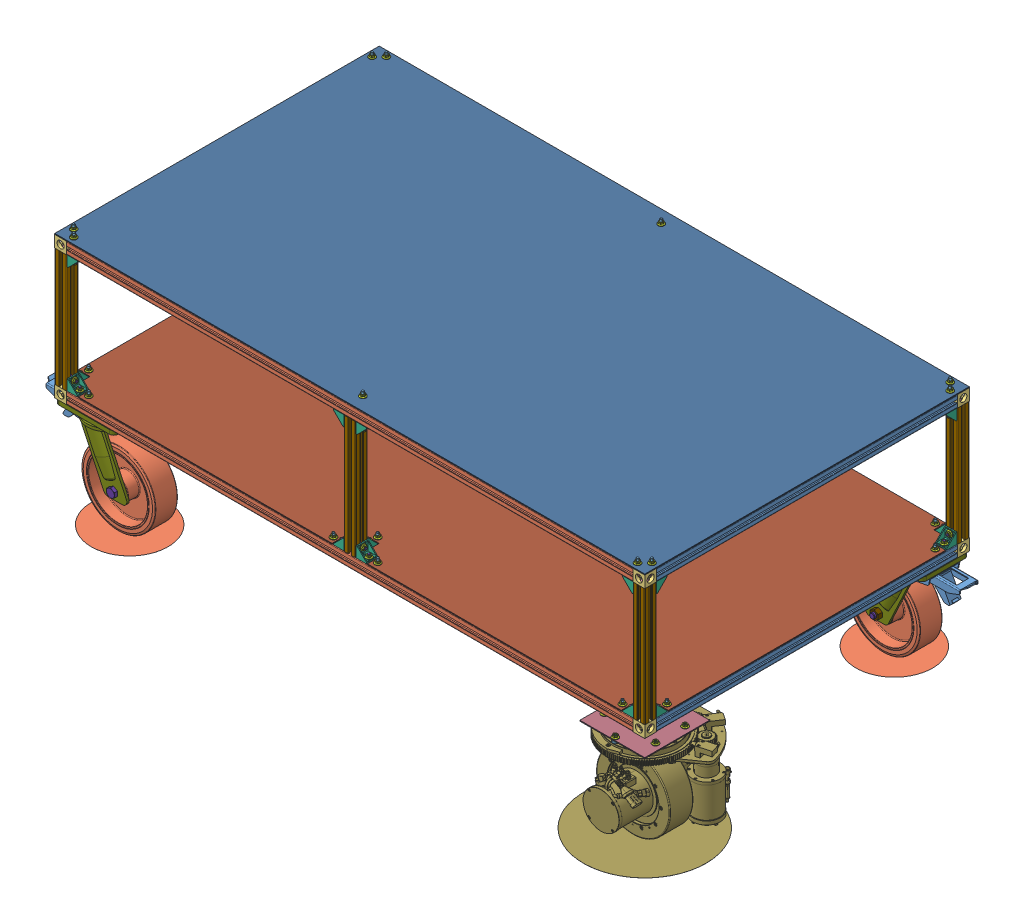
SolidWorks assembly totale, configuration Default. Lengths in mm.
Overall size (2298.39 831.64 1387.9).
545 component instances, 20 part files, 36 mates.
Components (placement in the parent):
- body-1: body [Default] at (-233.7628 101.484 2240) size (2000 498.7 1100)
  - body_skeleton-1: body_skeleton [Default] at (-1.581 -195.357 0) size (2000 480 1100)
    - Piano_base-1: Piano_base [Default] at (1030.9122 10.7283 790) size (2000 66.8 1100)
      - profilato_1020-1: profilato_1020 [Default] at (-20 -20 -1540) size (40 40 1020)
      - profilato_1920-1: profilato_1920 [Default] at (-40 -20 -1560) x (0 1 0) z (-1 0 0) size (40 40 1920)
      - profilato_1020-2: profilato_1020 [Default] at (-1980 -20 -520) x (0 -1 0) z (0 0 -1) size (40 40 1020)
      - profilato_1920-2: profilato_1920 [Default] at (-40 -20 -500) x (0 0 -1) z (-1 0 0) size (40 40 1920)
      - cubic_joint_screws-1: cubic_joint_screws [Default] at (-11.6556 -20 -1565.4929) x (0 0 1) z (0 -1 0) size (66.8 66.8 66.8)
        - cubic_joint_3-1: cubic_joint_3 [Default] at (25.4929 8.3444 0) size (40 40 40)
        - CORE_SCREW_S12X30_T50-1: CORE_SCREW_S12X30_T50 [Default] at (27.9929 8.3444 0) x (0 -0.924225 -0.381849) z (1 0 0) size (19.6 19.6 35.7)
        - CORE_SCREW_S12X30_T50-2: CORE_SCREW_S12X30_T50 [Default] at (5.4929 30.8444 0) x (-0.999796 0 0.020189) z (0 1 0) size (19.6 19.6 35.7)
        - CORE_SCREW_S12X30_T50-3: CORE_SCREW_S12X30_T50 [Default] at (5.4929 8.3444 -22.5) x (-0.923728 -0.383049 0) z (0 0 -1) size (19.6 19.6 35.7)
      - cubic_joint_screws-2: cubic_joint_screws [Default] at (-1985.4929 -20 -1568.3444) x (1 0 0) z (0 -1 0) size (66.8 66.8 66.8)
        - cubic_joint_3-1: cubic_joint_3 [Default] at (25.4929 8.3444 0) size (40 40 40)
        - CORE_SCREW_S12X30_T50-1: CORE_SCREW_S12X30_T50 [Default] at (27.9929 8.3444 0) x (0 -0.924225 -0.381849) z (1 0 0) size (19.6 19.6 35.7)
        - CORE_SCREW_S12X30_T50-2: CORE_SCREW_S12X30_T50 [Default] at (5.4929 30.8444 0) x (-0.999796 0 0.020189) z (0 1 0) size (19.6 19.6 35.7)
        - CORE_SCREW_S12X30_T50-3: CORE_SCREW_S12X30_T50 [Default] at (5.4929 8.3444 -22.5) x (-0.923728 -0.383049 0) z (0 0 -1) size (19.6 19.6 35.7)
      - cubic_joint_screws-3: cubic_joint_screws [Default] at (-11.6556 -25.4929 -500) x (0 1 0) z (0 0 1) size (66.8 66.8 66.8)
        - cubic_joint_3-1: cubic_joint_3 [Default] at (25.4929 8.3444 0) size (40 40 40)
        - CORE_SCREW_S12X30_T50-1: CORE_SCREW_S12X30_T50 [Default] at (27.9929 8.3444 0) x (0 -0.924225 -0.381849) z (1 0 0) size (19.6 19.6 35.7)
        - CORE_SCREW_S12X30_T50-2: CORE_SCREW_S12X30_T50 [Default] at (5.4929 30.8444 0) x (-0.999796 0 0.020189) z (0 1 0) size (19.6 19.6 35.7)
        - CORE_SCREW_S12X30_T50-3: CORE_SCREW_S12X30_T50 [Default] at (5.4929 8.3444 -22.5) x (-0.923728 -0.383049 0) z (0 0 -1) size (19.6 19.6 35.7)
      - cubic_joint_screws-4: cubic_joint_screws [Default] at (-1985.4929 -28.3444 -500) size (66.8 66.8 66.8)
        - cubic_joint_3-1: cubic_joint_3 [Default] at (25.4929 8.3444 0) size (40 40 40)
        - CORE_SCREW_S12X30_T50-1: CORE_SCREW_S12X30_T50 [Default] at (27.9929 8.3444 0) x (0 -0.924225 -0.381849) z (1 0 0) size (19.6 19.6 35.7)
        - CORE_SCREW_S12X30_T50-2: CORE_SCREW_S12X30_T50 [Default] at (5.4929 30.8444 0) x (-0.999796 0 0.020189) z (0 1 0) size (19.6 19.6 35.7)
        - CORE_SCREW_S12X30_T50-3: CORE_SCREW_S12X30_T50 [Default] at (5.4929 8.3444 -22.5) x (-0.923728 -0.383049 0) z (0 0 -1) size (19.6 19.6 35.7)
      - longherone_h-4: longherone_h [Default] at (-1507.1648 -11.1801 -790) size (112 40 1043.4)
        - profilato_1020-1: profilato_1020 [Default] at (33.8348 -8.8199 -750) size (40 40 1020)
        - T_BOLT-1: T_BOLT [Default] at (33.8348 -8.8199 276) x (0 -1 0) z (0 0 1) size (19.4 8.5 30.4)
        - T_BOLT-2: T_BOLT [Default] at (33.8348 -8.8199 -756) x (0 -1 0) z (0 0 -1) size (19.4 8.5 30.4)
        - Bracket_40_40_set-2: Bracket_40_40_set [Default] at (-7.7665 -12.3804 -732) x (0 1 0) z (0 0 1) size (38 47.7 51.56)
          - bracket_40_40-1: bracket_40_40 [Default] at (-15.4395 -1.6013 2) size (38 36 36)
          - FLANGE_NUT_M8-3: FLANGE_NUT_M8 [Default] at (3.5605 3.5487 -12.5) size (21 21 8)
          - T_BOLT_short-4: T_BOLT_short [Default] at (3.5605 3.5487 -24) x (-1 0 0) z (0 0 -1) size (19.4 8.5 26.9)
          - FLANGE_NUT_M8-4: FLANGE_NUT_M8 [Default] at (3.5605 -16.1013 7.15) x (0.797177 0 0.603746) z (0 1 0) size (21 21 8)
          - T_BOLT_short-5: T_BOLT_short [Default] at (3.5605 -27.6013 7.15) x (-1 0 0) z (0 -1 0) size (19.4 8.5 26.9)
        - Bracket_40_40_set-3: Bracket_40_40_set [Default] at (75.436 -5.2593 -732) x (0 -1 0) z (0 0 1) size (38 47.7 51.56)
          - bracket_40_40-1: bracket_40_40 [Default] at (-15.4395 -1.6013 2) size (38 36 36)
          - FLANGE_NUT_M8-3: FLANGE_NUT_M8 [Default] at (3.5605 3.5487 -12.5) size (21 21 8)
          - T_BOLT_short-4: T_BOLT_short [Default] at (3.5605 3.5487 -24) x (-1 0 0) z (0 0 -1) size (19.4 8.5 26.9)
          - FLANGE_NUT_M8-4: FLANGE_NUT_M8 [Default] at (3.5605 -16.1013 7.15) x (0.797177 0 0.603746) z (0 1 0) size (21 21 8)
          - T_BOLT_short-5: T_BOLT_short [Default] at (3.5605 -27.6013 7.15) x (-1 0 0) z (0 -1 0) size (19.4 8.5 26.9)
        - Bracket_40_40_set-4: Bracket_40_40_set [Default] at (75.436 -12.3804 252) x (0 1 0) z (0 0 -1) size (38 47.7 51.56)
          - bracket_40_40-1: bracket_40_40 [Default] at (-15.4395 -1.6013 2) size (38 36 36)
          - FLANGE_NUT_M8-3: FLANGE_NUT_M8 [Default] at (3.5605 3.5487 -12.5) size (21 21 8)
          - T_BOLT_short-4: T_BOLT_short [Default] at (3.5605 3.5487 -24) x (-1 0 0) z (0 0 -1) size (19.4 8.5 26.9)
          - FLANGE_NUT_M8-4: FLANGE_NUT_M8 [Default] at (3.5605 -16.1013 7.15) x (0.797177 0 0.603746) z (0 1 0) size (21 21 8)
          - T_BOLT_short-5: T_BOLT_short [Default] at (3.5605 -27.6013 7.15) x (-1 0 0) z (0 -1 0) size (19.4 8.5 26.9)
        - Bracket_40_40_set-5: Bracket_40_40_set [Default] at (-7.7665 -5.2593 252) x (0 -1 0) z (0 0 -1) size (38 47.7 51.56)
          - bracket_40_40-1: bracket_40_40 [Default] at (-15.4395 -1.6013 2) size (38 36 36)
          - FLANGE_NUT_M8-3: FLANGE_NUT_M8 [Default] at (3.5605 3.5487 -12.5) size (21 21 8)
          - T_BOLT_short-4: T_BOLT_short [Default] at (3.5605 3.5487 -24) x (-1 0 0) z (0 0 -1) size (19.4 8.5 26.9)
          - FLANGE_NUT_M8-4: FLANGE_NUT_M8 [Default] at (3.5605 -16.1013 7.15) x (0.797177 0 0.603746) z (0 1 0) size (21 21 8)
          - T_BOLT_short-5: T_BOLT_short [Default] at (3.5605 -27.6013 7.15) x (-1 0 0) z (0 -1 0) size (19.4 8.5 26.9)
      - longherone_h-5: longherone_h [Default] at (-1033.8348 -11.1801 -790) size (112 40 1043.4)
        - profilato_1020-1: profilato_1020 [Default] at (33.8348 -8.8199 -750) size (40 40 1020)
        - T_BOLT-1: T_BOLT [Default] at (33.8348 -8.8199 276) x (0 -1 0) z (0 0 1) size (19.4 8.5 30.4)
        - T_BOLT-2: T_BOLT [Default] at (33.8348 -8.8199 -756) x (0 -1 0) z (0 0 -1) size (19.4 8.5 30.4)
        - Bracket_40_40_set-2: Bracket_40_40_set [Default] at (-7.7665 -12.3804 -732) x (0 1 0) z (0 0 1) size (38 47.7 51.56)
          - bracket_40_40-1: bracket_40_40 [Default] at (-15.4395 -1.6013 2) size (38 36 36)
          - FLANGE_NUT_M8-3: FLANGE_NUT_M8 [Default] at (3.5605 3.5487 -12.5) size (21 21 8)
          - T_BOLT_short-4: T_BOLT_short [Default] at (3.5605 3.5487 -24) x (-1 0 0) z (0 0 -1) size (19.4 8.5 26.9)
          - FLANGE_NUT_M8-4: FLANGE_NUT_M8 [Default] at (3.5605 -16.1013 7.15) x (0.797177 0 0.603746) z (0 1 0) size (21 21 8)
          - T_BOLT_short-5: T_BOLT_short [Default] at (3.5605 -27.6013 7.15) x (-1 0 0) z (0 -1 0) size (19.4 8.5 26.9)
        - Bracket_40_40_set-3: Bracket_40_40_set [Default] at (75.436 -5.2593 -732) x (0 -1 0) z (0 0 1) size (38 47.7 51.56)
          - bracket_40_40-1: bracket_40_40 [Default] at (-15.4395 -1.6013 2) size (38 36 36)
          - FLANGE_NUT_M8-3: FLANGE_NUT_M8 [Default] at (3.5605 3.5487 -12.5) size (21 21 8)
          - T_BOLT_short-4: T_BOLT_short [Default] at (3.5605 3.5487 -24) x (-1 0 0) z (0 0 -1) size (19.4 8.5 26.9)
          - FLANGE_NUT_M8-4: FLANGE_NUT_M8 [Default] at (3.5605 -16.1013 7.15) x (0.797177 0 0.603746) z (0 1 0) size (21 21 8)
          - T_BOLT_short-5: T_BOLT_short [Default] at (3.5605 -27.6013 7.15) x (-1 0 0) z (0 -1 0) size (19.4 8.5 26.9)
        - Bracket_40_40_set-4: Bracket_40_40_set [Default] at (75.436 -12.3804 252) x (0 1 0) z (0 0 -1) size (38 47.7 51.56)
          - bracket_40_40-1: bracket_40_40 [Default] at (-15.4395 -1.6013 2) size (38 36 36)
          - FLANGE_NUT_M8-3: FLANGE_NUT_M8 [Default] at (3.5605 3.5487 -12.5) size (21 21 8)
          - T_BOLT_short-4: T_BOLT_short [Default] at (3.5605 3.5487 -24) x (-1 0 0) z (0 0 -1) size (19.4 8.5 26.9)
          - FLANGE_NUT_M8-4: FLANGE_NUT_M8 [Default] at (3.5605 -16.1013 7.15) x (0.797177 0 0.603746) z (0 1 0) size (21 21 8)
          - T_BOLT_short-5: T_BOLT_short [Default] at (3.5605 -27.6013 7.15) x (-1 0 0) z (0 -1 0) size (19.4 8.5 26.9)
        - Bracket_40_40_set-5: Bracket_40_40_set [Default] at (-7.7665 -5.2593 252) x (0 -1 0) z (0 0 -1) size (38 47.7 51.56)
          - bracket_40_40-1: bracket_40_40 [Default] at (-15.4395 -1.6013 2) size (38 36 36)
          - FLANGE_NUT_M8-3: FLANGE_NUT_M8 [Default] at (3.5605 3.5487 -12.5) size (21 21 8)
          - T_BOLT_short-4: T_BOLT_short [Default] at (3.5605 3.5487 -24) x (-1 0 0) z (0 0 -1) size (19.4 8.5 26.9)
          - FLANGE_NUT_M8-4: FLANGE_NUT_M8 [Default] at (3.5605 -16.1013 7.15) x (0.797177 0 0.603746) z (0 1 0) size (21 21 8)
          - T_BOLT_short-5: T_BOLT_short [Default] at (3.5605 -27.6013 7.15) x (-1 0 0) z (0 -1 0) size (19.4 8.5 26.9)
      - longherone_h-6: longherone_h [Default] at (-560.5014 -11.1801 -790) size (112 40 1043.4)
        - profilato_1020-1: profilato_1020 [Default] at (33.8348 -8.8199 -750) size (40 40 1020)
        - T_BOLT-1: T_BOLT [Default] at (33.8348 -8.8199 276) x (0 -1 0) z (0 0 1) size (19.4 8.5 30.4)
        - T_BOLT-2: T_BOLT [Default] at (33.8348 -8.8199 -756) x (0 -1 0) z (0 0 -1) size (19.4 8.5 30.4)
        - Bracket_40_40_set-2: Bracket_40_40_set [Default] at (-7.7665 -12.3804 -732) x (0 1 0) z (0 0 1) size (38 47.7 51.56)
          - bracket_40_40-1: bracket_40_40 [Default] at (-15.4395 -1.6013 2) size (38 36 36)
          - FLANGE_NUT_M8-3: FLANGE_NUT_M8 [Default] at (3.5605 3.5487 -12.5) size (21 21 8)
          - T_BOLT_short-4: T_BOLT_short [Default] at (3.5605 3.5487 -24) x (-1 0 0) z (0 0 -1) size (19.4 8.5 26.9)
          - FLANGE_NUT_M8-4: FLANGE_NUT_M8 [Default] at (3.5605 -16.1013 7.15) x (0.797177 0 0.603746) z (0 1 0) size (21 21 8)
          - T_BOLT_short-5: T_BOLT_short [Default] at (3.5605 -27.6013 7.15) x (-1 0 0) z (0 -1 0) size (19.4 8.5 26.9)
        - Bracket_40_40_set-3: Bracket_40_40_set [Default] at (75.436 -5.2593 -732) x (0 -1 0) z (0 0 1) size (38 47.7 51.56)
          - bracket_40_40-1: bracket_40_40 [Default] at (-15.4395 -1.6013 2) size (38 36 36)
          - FLANGE_NUT_M8-3: FLANGE_NUT_M8 [Default] at (3.5605 3.5487 -12.5) size (21 21 8)
          - T_BOLT_short-4: T_BOLT_short [Default] at (3.5605 3.5487 -24) x (-1 0 0) z (0 0 -1) size (19.4 8.5 26.9)
          - FLANGE_NUT_M8-4: FLANGE_NUT_M8 [Default] at (3.5605 -16.1013 7.15) x (0.797177 0 0.603746) z (0 1 0) size (21 21 8)
          - T_BOLT_short-5: T_BOLT_short [Default] at (3.5605 -27.6013 7.15) x (-1 0 0) z (0 -1 0) size (19.4 8.5 26.9)
        - Bracket_40_40_set-4: Bracket_40_40_set [Default] at (75.436 -12.3804 252) x (0 1 0) z (0 0 -1) size (38 47.7 51.56)
          - bracket_40_40-1: bracket_40_40 [Default] at (-15.4395 -1.6013 2) size (38 36 36)
          - FLANGE_NUT_M8-3: FLANGE_NUT_M8 [Default] at (3.5605 3.5487 -12.5) size (21 21 8)
          - T_BOLT_short-4: T_BOLT_short [Default] at (3.5605 3.5487 -24) x (-1 0 0) z (0 0 -1) size (19.4 8.5 26.9)
          - FLANGE_NUT_M8-4: FLANGE_NUT_M8 [Default] at (3.5605 -16.1013 7.15) x (0.797177 0 0.603746) z (0 1 0) size (21 21 8)
          - T_BOLT_short-5: T_BOLT_short [Default] at (3.5605 -27.6013 7.15) x (-1 0 0) z (0 -1 0) size (19.4 8.5 26.9)
        - Bracket_40_40_set-5: Bracket_40_40_set [Default] at (-7.7665 -5.2593 252) x (0 -1 0) z (0 0 -1) size (38 47.7 51.56)
          - bracket_40_40-1: bracket_40_40 [Default] at (-15.4395 -1.6013 2) size (38 36 36)
          - FLANGE_NUT_M8-3: FLANGE_NUT_M8 [Default] at (3.5605 3.5487 -12.5) size (21 21 8)
          - T_BOLT_short-4: T_BOLT_short [Default] at (3.5605 3.5487 -24) x (-1 0 0) z (0 0 -1) size (19.4 8.5 26.9)
          - FLANGE_NUT_M8-4: FLANGE_NUT_M8 [Default] at (3.5605 -16.1013 7.15) x (0.797177 0 0.603746) z (0 1 0) size (21 21 8)
          - T_BOLT_short-5: T_BOLT_short [Default] at (3.5605 -27.6013 7.15) x (-1 0 0) z (0 -1 0) size (19.4 8.5 26.9)
      - Bracket_40_40_set-1: Bracket_40_40_set [Default] at (-58 -23.5605 -541.6013) x (0 1 0) z (-1 0 0) size (38 47.7 51.56)
        - bracket_40_40-1: bracket_40_40 [Default] at (-15.4395 -1.6013 2) size (38 36 36)
        - FLANGE_NUT_M8-3: FLANGE_NUT_M8 [Default] at (3.5605 3.5487 -12.5) size (21 21 8)
        - T_BOLT_short-4: T_BOLT_short [Default] at (3.5605 3.5487 -24) x (-1 0 0) z (0 0 -1) size (19.4 8.5 26.9)
        - FLANGE_NUT_M8-4: FLANGE_NUT_M8 [Default] at (3.5605 -16.1013 7.15) x (0.797177 0 0.603746) z (0 1 0) size (21 21 8)
        - T_BOLT_short-5: T_BOLT_short [Default] at (3.5605 -27.6013 7.15) x (-1 0 0) z (0 -1 0) size (19.4 8.5 26.9)
      - Bracket_40_40_set-2: Bracket_40_40_set [Default] at (-1942 -16.4395 -541.6013) x (0 -1 0) z (1 0 0) size (38 47.7 51.56)
        - bracket_40_40-1: bracket_40_40 [Default] at (-15.4395 -1.6013 2) size (38 36 36)
        - FLANGE_NUT_M8-3: FLANGE_NUT_M8 [Default] at (3.5605 3.5487 -12.5) size (21 21 8)
        - T_BOLT_short-4: T_BOLT_short [Default] at (3.5605 3.5487 -24) x (-1 0 0) z (0 0 -1) size (19.4 8.5 26.9)
        - FLANGE_NUT_M8-4: FLANGE_NUT_M8 [Default] at (3.5605 -16.1013 7.15) x (0.797177 0 0.603746) z (0 1 0) size (21 21 8)
        - T_BOLT_short-5: T_BOLT_short [Default] at (3.5605 -27.6013 7.15) x (-1 0 0) z (0 -1 0) size (19.4 8.5 26.9)
      - Bracket_40_40_set-3: Bracket_40_40_set [Default] at (-58 -16.4395 -1518.3987) x (0 -1 0) z (-1 0 0) size (38 47.7 51.56)
        - bracket_40_40-1: bracket_40_40 [Default] at (-15.4395 -1.6013 2) size (38 36 36)
        - FLANGE_NUT_M8-3: FLANGE_NUT_M8 [Default] at (3.5605 3.5487 -12.5) size (21 21 8)
        - T_BOLT_short-4: T_BOLT_short [Default] at (3.5605 3.5487 -24) x (-1 0 0) z (0 0 -1) size (19.4 8.5 26.9)
        - FLANGE_NUT_M8-4: FLANGE_NUT_M8 [Default] at (3.5605 -16.1013 7.15) x (0.797177 0 0.603746) z (0 1 0) size (21 21 8)
        - T_BOLT_short-5: T_BOLT_short [Default] at (3.5605 -27.6013 7.15) x (-1 0 0) z (0 -1 0) size (19.4 8.5 26.9)
      - Bracket_40_40_set-4: Bracket_40_40_set [Default] at (-1938.3987 -16.4395 -1522) x (0 -1 0) z (0 0 1) size (38 47.7 51.56)
        - bracket_40_40-1: bracket_40_40 [Default] at (-15.4395 -1.6013 2) size (38 36 36)
        - FLANGE_NUT_M8-3: FLANGE_NUT_M8 [Default] at (3.5605 3.5487 -12.5) size (21 21 8)
        - T_BOLT_short-4: T_BOLT_short [Default] at (3.5605 3.5487 -24) x (-1 0 0) z (0 0 -1) size (19.4 8.5 26.9)
        - FLANGE_NUT_M8-4: FLANGE_NUT_M8 [Default] at (3.5605 -16.1013 7.15) x (0.797177 0 0.603746) z (0 1 0) size (21 21 8)
        - T_BOLT_short-5: T_BOLT_short [Default] at (3.5605 -27.6013 7.15) x (-1 0 0) z (0 -1 0) size (19.4 8.5 26.9)
    - profilato_400-1: profilato_400 [Default] at (-949.0878 10.7283 -770) x (-1 0 0) z (0 1 0) size (40 40 400)
    - profilato_400-2: profilato_400 [Default] at (-949.0878 410.7283 290) x (-1 0 0) z (0 -1 0) size (40 40 400)
    - profilato_400-3: profilato_400 [Default] at (1010.9122 410.7283 290) x (-1 0 0) z (0 -1 0) size (40 40 400)
    - profilato_400-4: profilato_400 [Default] at (1010.9122 410.7283 -770) x (-1 0 0) z (0 -1 0) size (40 40 400)
    - Bracket_40_40_set-1: Bracket_40_40_set [Default] at (972.9122 32.3295 286.4395) x (0 0 1) z (-1 0 0) size (38 47.7 51.56)
      - bracket_40_40-1: bracket_40_40 [Default] at (-15.4395 -1.6013 2) size (38 36 36)
      - FLANGE_NUT_M8-3: FLANGE_NUT_M8 [Default] at (3.5605 3.5487 -12.5) size (21 21 8)
      - T_BOLT_short-4: T_BOLT_short [Default] at (3.5605 3.5487 -24) x (-1 0 0) z (0 0 -1) size (19.4 8.5 26.9)
      - FLANGE_NUT_M8-4: FLANGE_NUT_M8 [Default] at (3.5605 -16.1013 7.15) x (0.797177 0 0.603746) z (0 1 0) size (21 21 8)
      - T_BOLT_short-5: T_BOLT_short [Default] at (3.5605 -27.6013 7.15) x (-1 0 0) z (0 -1 0) size (19.4 8.5 26.9)
    - T_BOLT_short-1: T_BOLT_short [Default] at (1010.9122 416.7283 244.85) x (-1 0 0) z (0 1 0) size (19.4 8.5 26.9)
    - FLANGE_NUT_M8-1: FLANGE_NUT_M8 [Default] at (1010.9122 385.5783 264.5) x (0.923728 0.383049 0) z (0 0 -1) size (21 21 8)
    - bracket_40_40-1: bracket_40_40 [Default] at (991.9122 390.7283 250) x (1 0 0) z (0 0 -1) size (38 36 36)
    - FLANGE_NUT_M8-2: FLANGE_NUT_M8 [Default] at (1010.9122 405.2283 244.85) x (0.997587 0 -0.069426) z (0 -1 0) size (21 21 8)
    - T_BOLT_short-2: T_BOLT_short [Default] at (1010.9122 385.5783 276) x (-1 0 0) z (0 0 1) size (19.4 8.5 26.9)
    - T_BOLT_short-3: T_BOLT_short [Default] at (965.7622 416.7283 -770) x (0 0 1) z (0 1 0) size (19.4 8.5 26.9)
    - FLANGE_NUT_M8-3: FLANGE_NUT_M8 [Default] at (985.4122 385.5783 -770) x (0 0 1) z (-1 0 0) size (21 21 8)
    - bracket_40_40-2: bracket_40_40 [Default] at (970.9122 390.7283 -751) x (0 0 -1) z (-1 0 0) size (38 36 36)
    - FLANGE_NUT_M8-4: FLANGE_NUT_M8 [Default] at (965.7622 405.2283 -770) x (-0.069426 0 -0.997587) z (0 -1 0) size (21 21 8)
    - T_BOLT_short-4: T_BOLT_short [Default] at (996.9122 385.5783 -770) x (0 0 1) z (1 0 0) size (19.4 8.5 26.9)
    - T_BOLT_short-5: T_BOLT_short [Default] at (965.7622 416.7283 290) x (0 0 1) z (0 1 0) size (19.4 8.5 26.9)
    - FLANGE_NUT_M8-5: FLANGE_NUT_M8 [Default] at (985.4122 385.5783 290) x (0 -0.924225 -0.381849) z (-1 0 0) size (21 21 8)
    - bracket_40_40-3: bracket_40_40 [Default] at (970.9122 390.7283 309) x (0 0 -1) z (-1 0 0) size (38 36 36)
    - FLANGE_NUT_M8-6: FLANGE_NUT_M8 [Default] at (965.7622 405.2283 290) x (0.069426 0 0.997587) z (0 -1 0) size (21 21 8)
    - T_BOLT_short-6: T_BOLT_short [Default] at (996.9122 385.5783 290) x (0 0 1) z (1 0 0) size (19.4 8.5 26.9)
    - T_BOLT_short-7: T_BOLT_short [Default] at (1010.9122 4.7283 244.85) x (1 0 0) z (0 -1 0) size (19.4 8.5 26.9)
    - FLANGE_NUT_M8-7: FLANGE_NUT_M8 [Default] at (1010.9122 35.8783 264.5) x (0.923728 0.383049 0) z (0 0 -1) size (21 21 8)
    - bracket_40_40-4: bracket_40_40 [Default] at (1029.9122 30.7283 250) x (-1 0 0) z (0 0 -1) size (38 36 36)
    - FLANGE_NUT_M8-8: FLANGE_NUT_M8 [Default] at (1010.9122 16.2283 244.85) x (0.797177 0 0.603746) z (0 1 0) size (21 21 8)
    - T_BOLT_short-8: T_BOLT_short [Default] at (1010.9122 35.8783 276) size (19.4 8.5 26.9)
    - T_BOLT_short-9: T_BOLT_short [Default] at (996.9122 35.8783 -770) x (0 0 1) z (1 0 0) size (19.4 8.5 26.9)
    - FLANGE_NUT_M8-9: FLANGE_NUT_M8 [Default] at (965.7622 16.2283 -770) x (1 0 0) z (0 1 0) size (21 21 8)
    - bracket_40_40-5: bracket_40_40 [Default] at (970.9122 30.7283 -751) x (0 0 -1) z (0 1 0) size (38 36 36)
    - FLANGE_NUT_M8-10: FLANGE_NUT_M8 [Default] at (985.4122 35.8783 -770) x (0 0.351186 -0.936306) z (-1 0 0) size (21 21 8)
    - T_BOLT_short-10: T_BOLT_short [Default] at (965.7622 4.7283 -770) x (0 0 1) z (0 -1 0) size (19.4 8.5 26.9)
    - T_BOLT_short-11: T_BOLT_short [Default] at (1010.9122 4.7283 -724.85) x (-1 0 0) z (0 -1 0) size (19.4 8.5 26.9)
    - FLANGE_NUT_M8-11: FLANGE_NUT_M8 [Default] at (1010.9122 35.8783 -744.5) size (21 21 8)
    - bracket_40_40-6: bracket_40_40 [Default] at (991.9122 30.7283 -730) size (38 36 36)
    - FLANGE_NUT_M8-12: FLANGE_NUT_M8 [Default] at (1010.9122 16.2283 -724.85) x (0.797177 0 0.603746) z (0 1 0) size (21 21 8)
    - T_BOLT_short-12: T_BOLT_short [Default] at (1010.9122 35.8783 -756) x (-1 0 0) z (0 0 -1) size (19.4 8.5 26.9)
    - T_BOLT_short-13: T_BOLT_short [Default] at (1010.9122 416.7283 -724.85) x (1 0 0) z (0 1 0) size (19.4 8.5 26.9)
    - FLANGE_NUT_M8-13: FLANGE_NUT_M8 [Default] at (1010.9122 385.5783 -744.5) size (21 21 8)
    - bracket_40_40-7: bracket_40_40 [Default] at (1029.9122 390.7283 -730) x (-1 0 0) z (0 0 1) size (38 36 36)
    - FLANGE_NUT_M8-14: FLANGE_NUT_M8 [Default] at (1010.9122 405.2283 -724.85) x (0.997587 0 -0.069426) z (0 -1 0) size (21 21 8)
    - T_BOLT_short-14: T_BOLT_short [Default] at (1010.9122 385.5783 -756) x (1 0 0) z (0 0 -1) size (19.4 8.5 26.9)
    - T_BOLT_short-15: T_BOLT_short [Default] at (-903.9378 416.7283 -770) x (0 0 -1) z (0 1 0) size (19.4 8.5 26.9)
    - FLANGE_NUT_M8-15: FLANGE_NUT_M8 [Default] at (-923.5878 385.5783 -770) x (0 0 -1) z (1 0 0) size (21 21 8)
    - bracket_40_40-8: bracket_40_40 [Default] at (-909.0878 390.7283 -789) x (0 0 1) z (1 0 0) size (38 36 36)
    - FLANGE_NUT_M8-16: FLANGE_NUT_M8 [Default] at (-903.9378 405.2283 -770) x (0.069426 0 0.997587) z (0 -1 0) size (21 21 8)
    - T_BOLT_short-16: T_BOLT_short [Default] at (-935.0878 385.5783 -770) x (0 0 -1) z (-1 0 0) size (19.4 8.5 26.9)
    - T_BOLT_short-17: T_BOLT_short [Default] at (-949.0878 416.7283 -724.85) x (1 0 0) z (0 1 0) size (19.4 8.5 26.9)
    - FLANGE_NUT_M8-17: FLANGE_NUT_M8 [Default] at (-949.0878 385.5783 -744.5) size (21 21 8)
    - bracket_40_40-9: bracket_40_40 [Default] at (-930.0878 390.7283 -730) x (-1 0 0) z (0 0 1) size (38 36 36)
    - FLANGE_NUT_M8-18: FLANGE_NUT_M8 [Default] at (-949.0878 405.2283 -724.85) x (0.997587 0 -0.069426) z (0 -1 0) size (21 21 8)
    - T_BOLT_short-18: T_BOLT_short [Default] at (-949.0878 385.5783 -756) x (1 0 0) z (0 0 -1) size (19.4 8.5 26.9)
    - T_BOLT_short-19: T_BOLT_short [Default] at (-903.9378 4.7283 -770) x (0 0 1) z (0 -1 0) size (19.4 8.5 26.9)
    - FLANGE_NUT_M8-19: FLANGE_NUT_M8 [Default] at (-923.5878 35.8783 -770) x (0 0 -1) z (1 0 0) size (21 21 8)
    - bracket_40_40-10: bracket_40_40 [Default] at (-909.0878 30.7283 -751) x (0 0 -1) z (1 0 0) size (38 36 36)
    - FLANGE_NUT_M8-20: FLANGE_NUT_M8 [Default] at (-903.9378 16.2283 -770) x (0.603746 0 -0.797177) z (0 1 0) size (21 21 8)
    - T_BOLT_short-20: T_BOLT_short [Default] at (-935.0878 35.8783 -770) x (0 0 1) z (-1 0 0) size (19.4 8.5 26.9)
    - T_BOLT_short-21: T_BOLT_short [Default] at (-949.0878 4.7283 -724.85) x (-1 0 0) z (0 -1 0) size (19.4 8.5 26.9)
    - FLANGE_NUT_M8-21: FLANGE_NUT_M8 [Default] at (-949.0878 35.8783 -744.5) size (21 21 8)
    - bracket_40_40-11: bracket_40_40 [Default] at (-968.0878 30.7283 -730) size (38 36 36)
    - FLANGE_NUT_M8-22: FLANGE_NUT_M8 [Default] at (-949.0878 16.2283 -724.85) x (0.797177 0 0.603746) z (0 1 0) size (21 21 8)
    - T_BOLT_short-22: T_BOLT_short [Default] at (-949.0878 35.8783 -756) x (-1 0 0) z (0 0 -1) size (19.4 8.5 26.9)
    - T_BOLT_short-23: T_BOLT_short [Default] at (-949.0878 4.7283 244.85) x (1 0 0) z (0 -1 0) size (19.4 8.5 26.9)
    - FLANGE_NUT_M8-23: FLANGE_NUT_M8 [Default] at (-949.0878 35.8783 264.5) x (0.923728 0.383049 0) z (0 0 -1) size (21 21 8)
    - bracket_40_40-12: bracket_40_40 [Default] at (-930.0878 30.7283 250) x (-1 0 0) z (0 0 -1) size (38 36 36)
    - FLANGE_NUT_M8-24: FLANGE_NUT_M8 [Default] at (-949.0878 16.2283 244.85) x (0.797177 0 0.603746) z (0 1 0) size (21 21 8)
    - T_BOLT_short-24: T_BOLT_short [Default] at (-949.0878 35.8783 276) size (19.4 8.5 26.9)
    - T_BOLT_short-25: T_BOLT_short [Default] at (-903.9378 4.7283 290) x (0 0 1) z (0 -1 0) size (19.4 8.5 26.9)
    - FLANGE_NUT_M8-25: FLANGE_NUT_M8 [Default] at (-923.5878 35.8783 290) x (0 0.924225 0.381849) z (1 0 0) size (21 21 8)
    - bracket_40_40-13: bracket_40_40 [Default] at (-909.0878 30.7283 309) x (0 0 -1) z (1 0 0) size (38 36 36)
    - FLANGE_NUT_M8-26: FLANGE_NUT_M8 [Default] at (-903.9378 16.2283 290) x (-0.603746 0 0.797177) z (0 1 0) size (21 21 8)
    - T_BOLT_short-26: T_BOLT_short [Default] at (-935.0878 35.8783 290) x (0 0 1) z (-1 0 0) size (19.4 8.5 26.9)
    - T_BOLT_short-27: T_BOLT_short [Default] at (-903.9378 416.7283 290) x (0 0 -1) z (0 1 0) size (19.4 8.5 26.9)
    - FLANGE_NUT_M8-27: FLANGE_NUT_M8 [Default] at (-923.5878 385.5783 290) x (0 0.924225 0.381849) z (1 0 0) size (21 21 8)
    - bracket_40_40-14: bracket_40_40 [Default] at (-909.0878 390.7283 271) x (0 0 1) z (1 0 0) size (38 36 36)
    - FLANGE_NUT_M8-28: FLANGE_NUT_M8 [Default] at (-903.9378 405.2283 290) x (-0.069426 0 -0.997587) z (0 -1 0) size (21 21 8)
    - T_BOLT_short-28: T_BOLT_short [Default] at (-935.0878 385.5783 290) x (0 0 -1) z (-1 0 0) size (19.4 8.5 26.9)
    - T_BOLT_short-29: T_BOLT_short [Default] at (-949.0878 416.7283 244.85) x (-1 0 0) z (0 1 0) size (19.4 8.5 26.9)
    - FLANGE_NUT_M8-29: FLANGE_NUT_M8 [Default] at (-949.0878 385.5783 264.5) x (0.923728 0.383049 0) z (0 0 -1) size (21 21 8)
    - bracket_40_40-15: bracket_40_40 [Default] at (-968.0878 390.7283 250) x (1 0 0) z (0 0 -1) size (38 36 36)
    - FLANGE_NUT_M8-30: FLANGE_NUT_M8 [Default] at (-949.0878 405.2283 244.85) x (0.997587 0 -0.069426) z (0 -1 0) size (21 21 8)
    - T_BOLT_short-30: T_BOLT_short [Default] at (-949.0878 385.5783 276) x (-1 0 0) z (0 0 1) size (19.4 8.5 26.9)
    - T_BOLT_short-33: T_BOLT_short [Default] at (76.0622 416.7283 -770) x (0 0 -1) z (0 1 0) size (19.4 8.5 26.9)
    - FLANGE_NUT_M8-33: FLANGE_NUT_M8 [Default] at (56.4122 385.5783 -770) x (0 0 -1) z (1 0 0) size (21 21 8)
    - bracket_40_40-17: bracket_40_40 [Default] at (70.9122 390.7283 -789) x (0 0 1) z (1 0 0) size (38 36 36)
    - FLANGE_NUT_M8-34: FLANGE_NUT_M8 [Default] at (76.0622 405.2283 -770) x (0.997587 0 -0.069426) z (0 -1 0) size (21 21 8)
    - T_BOLT_short-34: T_BOLT_short [Default] at (44.9122 385.5783 -770) x (0 0 -1) z (-1 0 0) size (19.4 8.5 26.9)
    - T_BOLT_short-35: T_BOLT_short [Default] at (30.9122 4.7283 -724.85) x (-1 0 0) z (0 -1 0) size (19.4 8.5 26.9)
    - FLANGE_NUT_M8-35: FLANGE_NUT_M8 [Default] at (30.9122 35.8783 -744.5) size (21 21 8)
    - bracket_40_40-18: bracket_40_40 [Default] at (11.9122 30.7283 -730) size (38 36 36)
    - FLANGE_NUT_M8-36: FLANGE_NUT_M8 [Default] at (30.9122 16.2283 -724.85) x (0.797177 0 0.603746) z (0 1 0) size (21 21 8)
    - T_BOLT_short-36: T_BOLT_short [Default] at (30.9122 35.8783 -756) x (-1 0 0) z (0 0 -1) size (19.4 8.5 26.9)
    - FLANGE_NUT_M8-37: FLANGE_NUT_M8 [Default] at (56.4122 35.8783 290) x (0 0 -1) z (1 0 0) size (21 21 8)
    - T_BOLT_short-37: T_BOLT_short [Default] at (76.0622 4.7283 290) x (0 0 1) z (0 -1 0) size (19.4 8.5 26.9)
    - bracket_40_40-19: bracket_40_40 [Default] at (-9.0878 30.7283 271) x (0 0 1) z (-1 0 0) size (38 36 36)
    - FLANGE_NUT_M8-38: FLANGE_NUT_M8 [Default] at (5.4122 35.8783 290) x (0 -0.924225 -0.381849) z (-1 0 0) size (21 21 8)
    - FLANGE_NUT_M8-39: FLANGE_NUT_M8 [Default] at (76.0622 16.2283 290) x (0.603746 0 -0.797177) z (0 1 0) size (21 21 8)
    - bracket_40_40-20: bracket_40_40 [Default] at (70.9122 30.7283 309) x (0 0 -1) z (1 0 0) size (38 36 36)
    - T_BOLT_short-38: T_BOLT_short [Default] at (16.9122 35.8783 290) x (0 0 -1) z (1 0 0) size (19.4 8.5 26.9)
    - T_BOLT_short-39: T_BOLT_short [Default] at (-14.2378 4.7283 290) x (0 0 -1) z (0 -1 0) size (19.4 8.5 26.9)
    - FLANGE_NUT_M8-40: FLANGE_NUT_M8 [Default] at (-14.2378 16.2283 290) x (0.603746 0 -0.797177) z (0 1 0) size (21 21 8)
    - T_BOLT_short-40: T_BOLT_short [Default] at (44.9122 35.8783 290) x (0 0 1) z (-1 0 0) size (19.4 8.5 26.9)
    - T_BOLT_short-41: T_BOLT_short [Default] at (44.9122 385.5783 290) x (0 0 -1) z (-1 0 0) size (19.4 8.5 26.9)
    - FLANGE_NUT_M8-41: FLANGE_NUT_M8 [Default] at (-14.2378 405.2283 290) x (0.997587 0 -0.069426) z (0 -1 0) size (21 21 8)
    - T_BOLT_short-42: T_BOLT_short [Default] at (16.9122 385.5783 290) x (0 0 1) z (1 0 0) size (19.4 8.5 26.9)
    - FLANGE_NUT_M8-42: FLANGE_NUT_M8 [Default] at (76.0622 405.2283 290) x (0.997587 0 -0.069426) z (0 -1 0) size (21 21 8)
    - FLANGE_NUT_M8-43: FLANGE_NUT_M8 [Default] at (5.4122 385.5783 290) x (0 0 1) z (-1 0 0) size (21 21 8)
    - FLANGE_NUT_M8-44: FLANGE_NUT_M8 [Default] at (56.4122 35.8783 -770) x (0 0 -1) z (1 0 0) size (21 21 8)
    - T_BOLT_short-43: T_BOLT_short [Default] at (76.0622 4.7283 -770) x (0 0 1) z (0 -1 0) size (19.4 8.5 26.9)
    - T_BOLT_short-44: T_BOLT_short [Default] at (76.0622 416.7283 290) x (0 0 -1) z (0 1 0) size (19.4 8.5 26.9)
    - bracket_40_40-21: bracket_40_40 [Default] at (49.9122 30.7283 250) x (-1 0 0) z (0 0 -1) size (38 36 36)
    - bracket_40_40-22: bracket_40_40 [Default] at (70.9122 390.7283 271) x (0 0 1) z (1 0 0) size (38 36 36)
    - FLANGE_NUT_M8-45: FLANGE_NUT_M8 [Default] at (30.9122 35.8783 264.5) x (0.923728 0.383049 0) z (0 0 -1) size (21 21 8)
    - bracket_40_40-23: bracket_40_40 [Default] at (-9.0878 390.7283 309) x (0 0 -1) z (-1 0 0) size (38 36 36)
    - FLANGE_NUT_M8-46: FLANGE_NUT_M8 [Default] at (76.0622 16.2283 -770) x (0.797177 0 0.603746) z (0 1 0) size (21 21 8)
    - bracket_40_40-24: bracket_40_40 [Default] at (70.9122 30.7283 -751) x (0 0 -1) z (1 0 0) size (38 36 36)
    - T_BOLT_short-45: T_BOLT_short [Default] at (30.9122 35.8783 276) size (19.4 8.5 26.9)
    - T_BOLT_short-46: T_BOLT_short [Default] at (30.9122 4.7283 244.85) x (1 0 0) z (0 -1 0) size (19.4 8.5 26.9)
    - T_BOLT_short-47: T_BOLT_short [Default] at (-14.2378 416.7283 290) x (0 0 1) z (0 1 0) size (19.4 8.5 26.9)
    - FLANGE_NUT_M8-47: FLANGE_NUT_M8 [Default] at (56.4122 385.5783 290) x (0 0 -1) z (1 0 0) size (21 21 8)
    - FLANGE_NUT_M8-48: FLANGE_NUT_M8 [Default] at (30.9122 16.2283 244.85) x (0.797177 0 0.603746) z (0 1 0) size (21 21 8)
    - T_BOLT_short-48: T_BOLT_short [Default] at (44.9122 35.8783 -770) x (0 0 1) z (-1 0 0) size (19.4 8.5 26.9)
    - T_BOLT_short-49: T_BOLT_short [Default] at (16.9122 385.5783 -770) x (0 0 1) z (1 0 0) size (19.4 8.5 26.9)
    - FLANGE_NUT_M8-49: FLANGE_NUT_M8 [Default] at (30.9122 405.2283 244.85) x (0.997587 0 -0.069426) z (0 -1 0) size (21 21 8)
    - T_BOLT_short-50: T_BOLT_short [Default] at (30.9122 385.5783 276) x (-1 0 0) z (0 0 1) size (19.4 8.5 26.9)
    - FLANGE_NUT_M8-50: FLANGE_NUT_M8 [Default] at (-14.2378 405.2283 -770) x (0.997587 0 -0.069426) z (0 -1 0) size (21 21 8)
    - FLANGE_NUT_M8-51: FLANGE_NUT_M8 [Default] at (30.9122 385.5783 264.5) x (0.923728 0.383049 0) z (0 0 -1) size (21 21 8)
    - FLANGE_NUT_M8-52: FLANGE_NUT_M8 [Default] at (5.4122 35.8783 -770) x (0 -0.924225 -0.381849) z (-1 0 0) size (21 21 8)
    - T_BOLT_short-51: T_BOLT_short [Default] at (-14.2378 4.7283 -770) x (0 0 -1) z (0 -1 0) size (19.4 8.5 26.9)
    - T_BOLT_short-52: T_BOLT_short [Default] at (-14.2378 416.7283 -770) x (0 0 1) z (0 1 0) size (19.4 8.5 26.9)
    - bracket_40_40-25: bracket_40_40 [Default] at (49.9122 390.7283 -730) x (-1 0 0) z (0 0 1) size (38 36 36)
    - bracket_40_40-26: bracket_40_40 [Default] at (-9.0878 390.7283 -751) x (0 0 -1) z (-1 0 0) size (38 36 36)
    - FLANGE_NUT_M8-53: FLANGE_NUT_M8 [Default] at (30.9122 385.5783 -744.5) size (21 21 8)
    - bracket_40_40-27: bracket_40_40 [Default] at (11.9122 390.7283 250) x (1 0 0) z (0 0 -1) size (38 36 36)
    - FLANGE_NUT_M8-54: FLANGE_NUT_M8 [Default] at (-14.2378 16.2283 -770) x (0.797177 0 0.603746) z (0 1 0) size (21 21 8)
    - bracket_40_40-28: bracket_40_40 [Default] at (-9.0878 30.7283 -789) x (0 0 1) z (-1 0 0) size (38 36 36)
    - T_BOLT_short-53: T_BOLT_short [Default] at (30.9122 385.5783 -756) x (1 0 0) z (0 0 -1) size (19.4 8.5 26.9)
    - T_BOLT_short-54: T_BOLT_short [Default] at (30.9122 416.7283 -724.85) x (1 0 0) z (0 1 0) size (19.4 8.5 26.9)
    - T_BOLT_short-55: T_BOLT_short [Default] at (30.9122 416.7283 244.85) x (-1 0 0) z (0 1 0) size (19.4 8.5 26.9)
    - FLANGE_NUT_M8-55: FLANGE_NUT_M8 [Default] at (5.4122 385.5783 -770) x (0 0 1) z (-1 0 0) size (21 21 8)
    - FLANGE_NUT_M8-56: FLANGE_NUT_M8 [Default] at (30.9122 405.2283 -724.85) x (0.997587 0 -0.069426) z (0 -1 0) size (21 21 8)
    - T_BOLT_short-56: T_BOLT_short [Default] at (16.9122 35.8783 -770) x (0 0 -1) z (1 0 0) size (19.4 8.5 26.9)
    - profilato_400-6: profilato_400 [Default] at (30.9122 10.7283 290) x (-1 0 0) z (0 1 0) size (40 40 400)
    - profilato_400-7: profilato_400 [Default] at (30.9122 10.7283 -770) x (-1 0 0) z (0 1 0) size (40 40 400)
    - Piano_base-2: Piano_base [Default] at (1030.9122 410.7283 -1270) x (1 0 0) z (0 0 -1) size (2000 66.8 1100)
      - profilato_1020-1: profilato_1020 [Default] at (-20 -20 -1540) size (40 40 1020)
      - profilato_1920-1: profilato_1920 [Default] at (-40 -20 -1560) x (0 1 0) z (-1 0 0) size (40 40 1920)
      - profilato_1020-2: profilato_1020 [Default] at (-1980 -20 -520) x (0 -1 0) z (0 0 -1) size (40 40 1020)
      - profilato_1920-2: profilato_1920 [Default] at (-40 -20 -500) x (0 0 -1) z (-1 0 0) size (40 40 1920)
      - cubic_joint_screws-1: cubic_joint_screws [Default] at (-11.6556 -20 -1565.4929) x (0 0 1) z (0 -1 0) size (66.8 66.8 66.8)
        - cubic_joint_3-1: cubic_joint_3 [Default] at (25.4929 8.3444 0) size (40 40 40)
        - CORE_SCREW_S12X30_T50-1: CORE_SCREW_S12X30_T50 [Default] at (27.9929 8.3444 0) x (0 -0.924225 -0.381849) z (1 0 0) size (19.6 19.6 35.7)
        - CORE_SCREW_S12X30_T50-2: CORE_SCREW_S12X30_T50 [Default] at (5.4929 30.8444 0) x (-0.999796 0 0.020189) z (0 1 0) size (19.6 19.6 35.7)
        - CORE_SCREW_S12X30_T50-3: CORE_SCREW_S12X30_T50 [Default] at (5.4929 8.3444 -22.5) x (-0.923728 -0.383049 0) z (0 0 -1) size (19.6 19.6 35.7)
      - cubic_joint_screws-2: cubic_joint_screws [Default] at (-1985.4929 -20 -1568.3444) x (1 0 0) z (0 -1 0) size (66.8 66.8 66.8)
        - cubic_joint_3-1: cubic_joint_3 [Default] at (25.4929 8.3444 0) size (40 40 40)
        - CORE_SCREW_S12X30_T50-1: CORE_SCREW_S12X30_T50 [Default] at (27.9929 8.3444 0) x (0 -0.924225 -0.381849) z (1 0 0) size (19.6 19.6 35.7)
        - CORE_SCREW_S12X30_T50-2: CORE_SCREW_S12X30_T50 [Default] at (5.4929 30.8444 0) x (-0.999796 0 0.020189) z (0 1 0) size (19.6 19.6 35.7)
        - CORE_SCREW_S12X30_T50-3: CORE_SCREW_S12X30_T50 [Default] at (5.4929 8.3444 -22.5) x (-0.923728 -0.383049 0) z (0 0 -1) size (19.6 19.6 35.7)
      - cubic_joint_screws-3: cubic_joint_screws [Default] at (-11.6556 -25.4929 -500) x (0 1 0) z (0 0 1) size (66.8 66.8 66.8)
        - cubic_joint_3-1: cubic_joint_3 [Default] at (25.4929 8.3444 0) size (40 40 40)
        - CORE_SCREW_S12X30_T50-1: CORE_SCREW_S12X30_T50 [Default] at (27.9929 8.3444 0) x (0 -0.924225 -0.381849) z (1 0 0) size (19.6 19.6 35.7)
        - CORE_SCREW_S12X30_T50-2: CORE_SCREW_S12X30_T50 [Default] at (5.4929 30.8444 0) x (-0.999796 0 0.020189) z (0 1 0) size (19.6 19.6 35.7)
        - CORE_SCREW_S12X30_T50-3: CORE_SCREW_S12X30_T50 [Default] at (5.4929 8.3444 -22.5) x (-0.923728 -0.383049 0) z (0 0 -1) size (19.6 19.6 35.7)
      - cubic_joint_screws-4: cubic_joint_screws [Default] at (-1985.4929 -28.3444 -500) size (66.8 66.8 66.8)
        - cubic_joint_3-1: cubic_joint_3 [Default] at (25.4929 8.3444 0) size (40 40 40)
        - CORE_SCREW_S12X30_T50-1: CORE_SCREW_S12X30_T50 [Default] at (27.9929 8.3444 0) x (0 -0.924225 -0.381849) z (1 0 0) size (19.6 19.6 35.7)
        - CORE_SCREW_S12X30_T50-2: CORE_SCREW_S12X30_T50 [Default] at (5.4929 30.8444 0) x (-0.999796 0 0.020189) z (0 1 0) size (19.6 19.6 35.7)
        - CORE_SCREW_S12X30_T50-3: CORE_SCREW_S12X30_T50 [Default] at (5.4929 8.3444 -22.5) x (-0.923728 -0.383049 0) z (0 0 -1) size (19.6 19.6 35.7)
      - longherone_h-4: longherone_h [Default] at (-1507.1648 -11.1801 -790) size (112 40 1043.4)
        - profilato_1020-1: profilato_1020 [Default] at (33.8348 -8.8199 -750) size (40 40 1020)
        - T_BOLT-1: T_BOLT [Default] at (33.8348 -8.8199 276) x (0 -1 0) z (0 0 1) size (19.4 8.5 30.4)
        - T_BOLT-2: T_BOLT [Default] at (33.8348 -8.8199 -756) x (0 -1 0) z (0 0 -1) size (19.4 8.5 30.4)
        - Bracket_40_40_set-2: Bracket_40_40_set [Default] at (-7.7665 -12.3804 -732) x (0 1 0) z (0 0 1) size (38 47.7 51.56)
          - bracket_40_40-1: bracket_40_40 [Default] at (-15.4395 -1.6013 2) size (38 36 36)
          - FLANGE_NUT_M8-3: FLANGE_NUT_M8 [Default] at (3.5605 3.5487 -12.5) size (21 21 8)
          - T_BOLT_short-4: T_BOLT_short [Default] at (3.5605 3.5487 -24) x (-1 0 0) z (0 0 -1) size (19.4 8.5 26.9)
          - FLANGE_NUT_M8-4: FLANGE_NUT_M8 [Default] at (3.5605 -16.1013 7.15) x (0.797177 0 0.603746) z (0 1 0) size (21 21 8)
          - T_BOLT_short-5: T_BOLT_short [Default] at (3.5605 -27.6013 7.15) x (-1 0 0) z (0 -1 0) size (19.4 8.5 26.9)
        - Bracket_40_40_set-3: Bracket_40_40_set [Default] at (75.436 -5.2593 -732) x (0 -1 0) z (0 0 1) size (38 47.7 51.56)
          - bracket_40_40-1: bracket_40_40 [Default] at (-15.4395 -1.6013 2) size (38 36 36)
          - FLANGE_NUT_M8-3: FLANGE_NUT_M8 [Default] at (3.5605 3.5487 -12.5) size (21 21 8)
          - T_BOLT_short-4: T_BOLT_short [Default] at (3.5605 3.5487 -24) x (-1 0 0) z (0 0 -1) size (19.4 8.5 26.9)
          - FLANGE_NUT_M8-4: FLANGE_NUT_M8 [Default] at (3.5605 -16.1013 7.15) x (0.797177 0 0.603746) z (0 1 0) size (21 21 8)
          - T_BOLT_short-5: T_BOLT_short [Default] at (3.5605 -27.6013 7.15) x (-1 0 0) z (0 -1 0) size (19.4 8.5 26.9)
        - Bracket_40_40_set-4: Bracket_40_40_set [Default] at (75.436 -12.3804 252) x (0 1 0) z (0 0 -1) size (38 47.7 51.56)
          - bracket_40_40-1: bracket_40_40 [Default] at (-15.4395 -1.6013 2) size (38 36 36)
          - FLANGE_NUT_M8-3: FLANGE_NUT_M8 [Default] at (3.5605 3.5487 -12.5) size (21 21 8)
          - T_BOLT_short-4: T_BOLT_short [Default] at (3.5605 3.5487 -24) x (-1 0 0) z (0 0 -1) size (19.4 8.5 26.9)
          - FLANGE_NUT_M8-4: FLANGE_NUT_M8 [Default] at (3.5605 -16.1013 7.15) x (0.797177 0 0.603746) z (0 1 0) size (21 21 8)
          - T_BOLT_short-5: T_BOLT_short [Default] at (3.5605 -27.6013 7.15) x (-1 0 0) z (0 -1 0) size (19.4 8.5 26.9)
        - Bracket_40_40_set-5: Bracket_40_40_set [Default] at (-7.7665 -5.2593 252) x (0 -1 0) z (0 0 -1) size (38 47.7 51.56)
          - bracket_40_40-1: bracket_40_40 [Default] at (-15.4395 -1.6013 2) size (38 36 36)
          - FLANGE_NUT_M8-3: FLANGE_NUT_M8 [Default] at (3.5605 3.5487 -12.5) size (21 21 8)
          - T_BOLT_short-4: T_BOLT_short [Default] at (3.5605 3.5487 -24) x (-1 0 0) z (0 0 -1) size (19.4 8.5 26.9)
          - FLANGE_NUT_M8-4: FLANGE_NUT_M8 [Default] at (3.5605 -16.1013 7.15) x (0.797177 0 0.603746) z (0 1 0) size (21 21 8)
          - T_BOLT_short-5: T_BOLT_short [Default] at (3.5605 -27.6013 7.15) x (-1 0 0) z (0 -1 0) size (19.4 8.5 26.9)
      - longherone_h-5: longherone_h [Default] at (-1033.8348 -11.1801 -790) size (112 40 1043.4)
        - profilato_1020-1: profilato_1020 [Default] at (33.8348 -8.8199 -750) size (40 40 1020)
        - T_BOLT-1: T_BOLT [Default] at (33.8348 -8.8199 276) x (0 -1 0) z (0 0 1) size (19.4 8.5 30.4)
        - T_BOLT-2: T_BOLT [Default] at (33.8348 -8.8199 -756) x (0 -1 0) z (0 0 -1) size (19.4 8.5 30.4)
        - Bracket_40_40_set-2: Bracket_40_40_set [Default] at (-7.7665 -12.3804 -732) x (0 1 0) z (0 0 1) size (38 47.7 51.56)
          - bracket_40_40-1: bracket_40_40 [Default] at (-15.4395 -1.6013 2) size (38 36 36)
          - FLANGE_NUT_M8-3: FLANGE_NUT_M8 [Default] at (3.5605 3.5487 -12.5) size (21 21 8)
          - T_BOLT_short-4: T_BOLT_short [Default] at (3.5605 3.5487 -24) x (-1 0 0) z (0 0 -1) size (19.4 8.5 26.9)
          - FLANGE_NUT_M8-4: FLANGE_NUT_M8 [Default] at (3.5605 -16.1013 7.15) x (0.797177 0 0.603746) z (0 1 0) size (21 21 8)
          - T_BOLT_short-5: T_BOLT_short [Default] at (3.5605 -27.6013 7.15) x (-1 0 0) z (0 -1 0) size (19.4 8.5 26.9)
        - Bracket_40_40_set-3: Bracket_40_40_set [Default] at (75.436 -5.2593 -732) x (0 -1 0) z (0 0 1) size (38 47.7 51.56)
          - bracket_40_40-1: bracket_40_40 [Default] at (-15.4395 -1.6013 2) size (38 36 36)
          - FLANGE_NUT_M8-3: FLANGE_NUT_M8 [Default] at (3.5605 3.5487 -12.5) size (21 21 8)
          - T_BOLT_short-4: T_BOLT_short [Default] at (3.5605 3.5487 -24) x (-1 0 0) z (0 0 -1) size (19.4 8.5 26.9)
          - FLANGE_NUT_M8-4: FLANGE_NUT_M8 [Default] at (3.5605 -16.1013 7.15) x (0.797177 0 0.603746) z (0 1 0) size (21 21 8)
          - T_BOLT_short-5: T_BOLT_short [Default] at (3.5605 -27.6013 7.15) x (-1 0 0) z (0 -1 0) size (19.4 8.5 26.9)
        - Bracket_40_40_set-4: Bracket_40_40_set [Default] at (75.436 -12.3804 252) x (0 1 0) z (0 0 -1) size (38 47.7 51.56)
          - bracket_40_40-1: bracket_40_40 [Default] at (-15.4395 -1.6013 2) size (38 36 36)
          - FLANGE_NUT_M8-3: FLANGE_NUT_M8 [Default] at (3.5605 3.5487 -12.5) size (21 21 8)
          - T_BOLT_short-4: T_BOLT_short [Default] at (3.5605 3.5487 -24) x (-1 0 0) z (0 0 -1) size (19.4 8.5 26.9)
          - FLANGE_NUT_M8-4: FLANGE_NUT_M8 [Default] at (3.5605 -16.1013 7.15) x (0.797177 0 0.603746) z (0 1 0) size (21 21 8)
          - T_BOLT_short-5: T_BOLT_short [Default] at (3.5605 -27.6013 7.15) x (-1 0 0) z (0 -1 0) size (19.4 8.5 26.9)
        - Bracket_40_40_set-5: Bracket_40_40_set [Default] at (-7.7665 -5.2593 252) x (0 -1 0) z (0 0 -1) size (38 47.7 51.56)
          - bracket_40_40-1: bracket_40_40 [Default] at (-15.4395 -1.6013 2) size (38 36 36)
          - FLANGE_NUT_M8-3: FLANGE_NUT_M8 [Default] at (3.5605 3.5487 -12.5) size (21 21 8)
          - T_BOLT_short-4: T_BOLT_short [Default] at (3.5605 3.5487 -24) x (-1 0 0) z (0 0 -1) size (19.4 8.5 26.9)
          - FLANGE_NUT_M8-4: FLANGE_NUT_M8 [Default] at (3.5605 -16.1013 7.15) x (0.797177 0 0.603746) z (0 1 0) size (21 21 8)
          - T_BOLT_short-5: T_BOLT_short [Default] at (3.5605 -27.6013 7.15) x (-1 0 0) z (0 -1 0) size (19.4 8.5 26.9)
